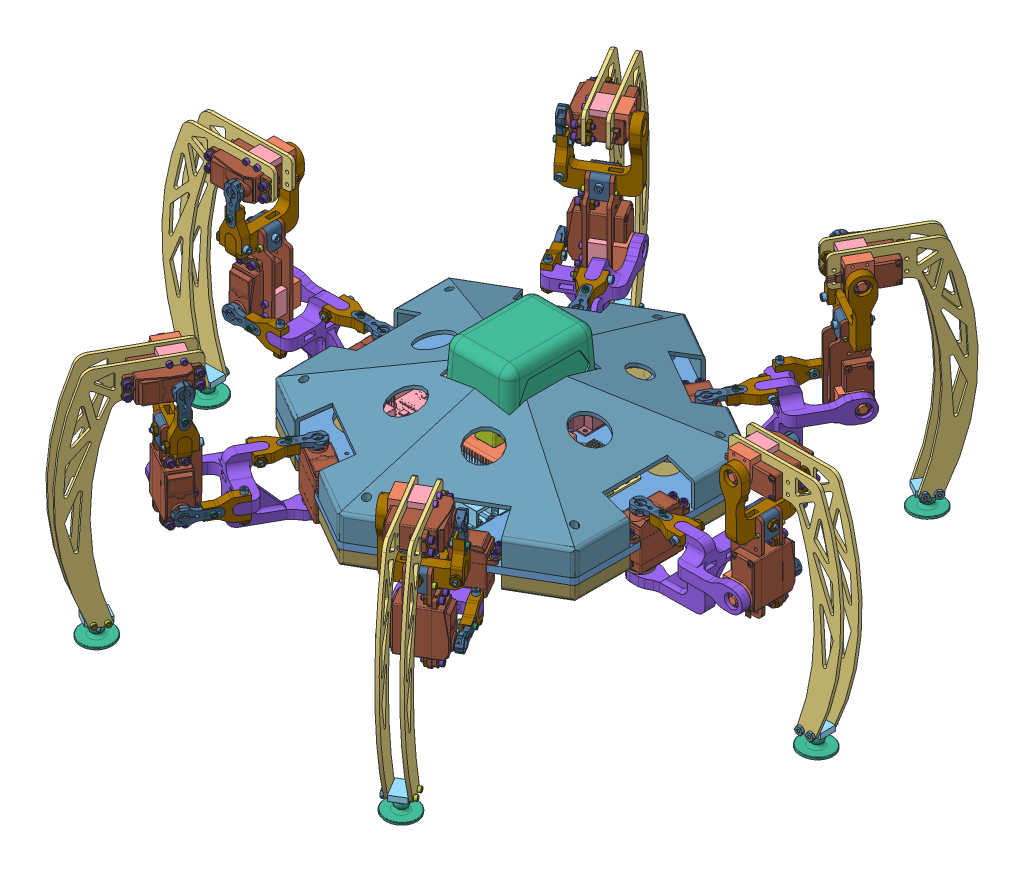
SolidWorks assembly Hexapod_(Hexagonal), configuration Défaut. Lengths in mm. (continued)
Components (placement in the parent): (continued)
- Foot+Tibia+Femur-11: Foot+Tibia+Femur [Défaut] at (-76.9411 -25 -93.0658) x (0.5 0 0.866025) z (-0.866025 0 0.5) size (210.19 223.27 63.83) (flexible)
  - Femur-1: Femur [Défaut] at origin size (137.43 61.64 61.08) (flexible)
    - Joint_(Femur_to_tibia)-1: Joint_(Femur_to_tibia) [Défaut] at (-66.4348 29.5 -48.8085) x (0.999924 0 -0.012321) z (0.012321 0 0.999924) size (122 58.8 58.8)
    - Horn_attachment-3: Horn_attachment [Défaut] at (-38.1979 44.8 -29.755) x (0.999924 0 -0.012321) z (0 1 0) size (33 20 8)
    - Horn-3: Horn [Défaut] at (-10.2 48.8 -30.1) x (-0.999924 0 0.012321) z (0 1 0) size (35.39 15.87 6)
    - DS3225MG-3: DS3225MG [Default] at (-10.2 45.8 -30.1) x (0 0 1) z (0 1 0) size (57.25 20.4 45.91)
    - Bearing_mount_(Femur)-1: Bearing_mount_(Femur) [Default] at (2.5 22 -30.1) x (1 0 0) z (0 -1 0) size (35.3 20.2 31)
    - Bearing-3: Bearing [Default] at (-10.2 -6.7498 -30.1) x (0.400474 0 0.916308) z (-0.916308 0 0.400474) size (13.87 4.75 13.87)
    - MSHXNUT 0.112-40-D-N-1: MSHXNUT 0.112-40-D-N [MSHXNUT 0.112-40-D-N] at (-30.1985 40.8 -29.8536) x (-0.510633 0 -0.859799) z (0 1 0) size (6.35 7.33 2.49)
    - HX-SHCS 0.112-40x0.4375x0.4375-N-1: HX-SHCS 0.112-40x0.4375x0.4375-N [HX-SHCS 0.112-40x0.4375x0.4375-N] at (-30.1985 51.6448 -29.8536) x (0 -1 0) z (-0.489292 0 0.87212) size (13.96 4.65 4.65)
    - Narrow FW 0.138-1: Narrow FW 0.138 [Narrow FW 0.138] at (-15.2 31.2 4.7) x (0 -1 0) z (-0.829316 0 -0.55878) size (0.81 7.92 7.92)
    - HX-SHCS 0.138-32x0.5x0.5-N-1: HX-SHCS 0.138-32x0.5x0.5-N [HX-SHCS 0.138-32x0.5x0.5-N] at (-15.2 35.772 4.7) x (0 -1 0) z (0.866025 0 -0.5) size (16.21 5.74 5.74)
    - Narrow FW 0.138-2: Narrow FW 0.138 [Narrow FW 0.138] at (-15.2 31.2 -44.9) x (0 -1 0) z (-0.829316 0 -0.55878) size (0.81 7.92 7.92)
    - Narrow FW 0.138-3: Narrow FW 0.138 [Narrow FW 0.138] at (-5.2 31.2 4.7) x (0 -1 0) z (-0.829316 0 -0.55878) size (0.81 7.92 7.92)
    - Narrow FW 0.138-4: Narrow FW 0.138 [Narrow FW 0.138] at (-5.2 31.2 -44.9) x (0 -1 0) z (-0.829316 0 -0.55878) size (0.81 7.92 7.92)
    - HX-SHCS 0.138-32x0.5x0.5-N-2: HX-SHCS 0.138-32x0.5x0.5-N [HX-SHCS 0.138-32x0.5x0.5-N] at (-15.2 35.772 -44.9) x (0 -1 0) z (0.866025 0 -0.5) size (16.21 5.74 5.74)
    - HX-SHCS 0.138-32x0.5x0.5-N-3: HX-SHCS 0.138-32x0.5x0.5-N [HX-SHCS 0.138-32x0.5x0.5-N] at (-5.2 35.772 4.7) x (0 -1 0) z (0.866025 0 -0.5) size (16.21 5.74 5.74)
    - HX-SHCS 0.138-32x0.5x0.5-N-4: HX-SHCS 0.138-32x0.5x0.5-N [HX-SHCS 0.138-32x0.5x0.5-N] at (-5.2 35.772 -44.9) x (0 -1 0) z (0.866025 0 -0.5) size (16.21 5.74 5.74)
    - MSHXNUT 0.138-32-D-N-1: MSHXNUT 0.138-32-D-N [MSHXNUT 0.138-32-D-N] at (-52.0379 44.8 -16.6879) x (-0.86596 -0.5 0.010671) z (0.012321 0 0.999924) size (7.92 9.15 2.9)
    - HX-SHCS 0.138-32x1x1-N-2: HX-SHCS 0.138-32x1x1-N [HX-SHCS 0.138-32x1x1-N] at (-52.3632 44.8 -43.0867) x (0.012321 0 0.999924) z (-0.86596 -0.5 0.010671) size (28.91 5.74 5.74)
  - Foot_(Long)-4: Foot_(Long) [Défaut] at (-141.7664 117.7478 -37.8795) x (0.999923 0.001668 -0.012321) z (0.012321 0 0.999924) size (104.1 223.13 60.64) (flexible)
    - DS3225MG-1: DS3225MG [Default] at (30.1 10.2 45.8) x (-1 0 0) z (0 0 1) size (57.25 20.4 45.91)
    - Bearing-1: Bearing [Default] at (30.1 10.2 -6.7498) x (-0.568255 0.822853 0) z (0.822853 0.568255 0) size (13.87 4.75 13.87)
    - Bearing_mount_(Foot)-1: Bearing_mount_(Foot) [Default] at (30.1 22.9 8.1) x (0 1 0) z (0 0 -1) size (25.3 20.2 17.1)
    - Foot_(Long)-1: Foot_(Long) [Default] at (18.7 14 25) size (103.08 208 3)
    - Link-1: Link [Default] at (30.1 22.9 11.1) x (0 -1 0) z (0 0 1) size (5 20.2 13.9)
    - Foot_(Long)-2: Foot_(Long) [Default] at (18.7 14 8.1) size (103.08 208 3)
    - Joint_(Foot_to_slipper)-2: Joint_(Foot_to_slipper) [Default] at (-21.9427 -177.5 11.1) x (0 1 0) z (0 0 1) size (15 20.2 13.9)
    - Horn-1: Horn [Défaut] at (30.1 10.2 48.8) x (-0.007987 -0.999968 0) z (0 0 1) size (35.39 15.87 6)
    - Horn_attachment-1: Horn_attachment [Défaut] at (29.8764 -17.7991 44.8) x (0.007987 0.999968 0) z (0 0 1) size (33 20 8)
    - Slipper-1: Slipper [Défaut] at (-21.7184 -191.9896 17.7406) x (0.999392 0.031392 0.015197) z (-0.013787 -0.044657 0.998907) size (30 10.55 30)
    - HX-SHCS 0.112-40x0.4375x0.4375-N-15: HX-SHCS 0.112-40x0.4375x0.4375-N [HX-SHCS 0.112-40x0.4375x0.4375-N] at (29.9403 -9.7994 51.6448) x (0 0 -1) z (0.869991 0.493067 0) size (13.96 4.65 4.65)
    - MSHXNUT 0.112-40-D-N-7: MSHXNUT 0.112-40-D-N [MSHXNUT 0.112-40-D-N] at (29.9403 -9.7994 40.8) x (-0.007987 -0.999968 0) z (0 0 1) size (6.35 7.33 2.49)
    - HX-SHCS 0.112-40x0.875x0.875-N-9: HX-SHCS 0.112-40x0.875x0.875-N [HX-SHCS 0.112-40x0.875x0.875-N] at (-26.9427 -177.5 30.8448) x (0 0 -1) z (0 1 0) size (25.07 4.65 4.65)
    - MSHXNUT 0.112-40-D-N-4: MSHXNUT 0.112-40-D-N [MSHXNUT 0.112-40-D-N] at (-26.9427 -177.5 8.1) x (0.866025 -0.5 0) z (0 0 1) size (6.35 7.33 2.49)
    - HX-SHCS 0.112-40x0.875x0.875-N-11: HX-SHCS 0.112-40x0.875x0.875-N [HX-SHCS 0.112-40x0.875x0.875-N] at (-16.9427 -177.5 30.8448) x (0 0 -1) z (0 1 0) size (25.07 4.65 4.65)
    - MSHXNUT 0.112-40-D-N-6: MSHXNUT 0.112-40-D-N [MSHXNUT 0.112-40-D-N] at (-16.9427 -177.5 8.1) x (0.866025 -0.5 0) z (0 0 1) size (6.35 7.33 2.49)
    - HX-SHCS 0.112-40x1x0.75-N-13: HX-SHCS 0.112-40x1x0.75-N [HX-SHCS 0.112-40x1x0.75-N] at (25.1 22.9 30.8448) x (0 0 -1) z (0 1 0) size (28.24 4.65 4.65)
    - HX-SHCS 0.112-40x1x0.75-N-14: HX-SHCS 0.112-40x1x0.75-N [HX-SHCS 0.112-40x1x0.75-N] at (35.1 22.9 30.8448) x (0 0 -1) z (0 1 0) size (28.24 4.65 4.65)
    - HX-SHCS 0.138-32x0.5x0.5-N-14: HX-SHCS 0.138-32x0.5x0.5-N [HX-SHCS 0.138-32x0.5x0.5-N] at (-4.7 5.2 35.772) x (0 0 -1) z (0.866025 0.5 0) size (16.21 5.74 5.74)
    - Narrow FW 0.138-1: Narrow FW 0.138 [Narrow FW 0.138] at (-4.7 5.2 31.2) x (0 0 -1) z (-0.829316 0.55878 0) size (0.81 7.92 7.92)
    - MSHXNUT 0.138-32-D-N-1: MSHXNUT 0.138-32-D-N [MSHXNUT 0.138-32-D-N] at (-4.7 5.2 25) x (0.866025 0.5 0) z (0 0 1) size (7.92 9.15 2.9)
    - MSHXNUT 0.138-32-D-N-2: MSHXNUT 0.138-32-D-N [MSHXNUT 0.138-32-D-N] at (44.9 5.2 25) x (0.866025 0.5 0) z (0 0 1) size (7.92 9.15 2.9)
    - MSHXNUT 0.138-32-D-N-3: MSHXNUT 0.138-32-D-N [MSHXNUT 0.138-32-D-N] at (-4.7 15.2 25) x (0.866025 0.5 0) z (0 0 1) size (7.92 9.15 2.9)
    - MSHXNUT 0.138-32-D-N-4: MSHXNUT 0.138-32-D-N [MSHXNUT 0.138-32-D-N] at (44.9 15.2 25) x (0.866025 0.5 0) z (0 0 1) size (7.92 9.15 2.9)
    - HX-SHCS 0.138-32x0.5x0.5-N-15: HX-SHCS 0.138-32x0.5x0.5-N [HX-SHCS 0.138-32x0.5x0.5-N] at (44.9 5.2 35.772) x (0 0 -1) z (0.866025 0.5 0) size (16.21 5.74 5.74)
    - HX-SHCS 0.138-32x0.5x0.5-N-16: HX-SHCS 0.138-32x0.5x0.5-N [HX-SHCS 0.138-32x0.5x0.5-N] at (-4.7 15.2 35.772) x (0 0 -1) z (0.866025 0.5 0) size (16.21 5.74 5.74)
    - HX-SHCS 0.138-32x0.5x0.5-N-17: HX-SHCS 0.138-32x0.5x0.5-N [HX-SHCS 0.138-32x0.5x0.5-N] at (44.9 15.2 35.772) x (0 0 -1) z (0.866025 0.5 0) size (16.21 5.74 5.74)
    - Narrow FW 0.138-2: Narrow FW 0.138 [Narrow FW 0.138] at (44.9 5.2 31.2) x (0 0 -1) z (-0.829316 0.55878 0) size (0.81 7.92 7.92)
    - Narrow FW 0.138-3: Narrow FW 0.138 [Narrow FW 0.138] at (-4.7 15.2 31.2) x (0 0 -1) z (-0.829316 0.55878 0) size (0.81 7.92 7.92)
    - Narrow FW 0.138-4: Narrow FW 0.138 [Narrow FW 0.138] at (44.9 15.2 31.2) x (0 0 -1) z (-0.829316 0.55878 0) size (0.81 7.92 7.92)
  - Tibia-3: Tibia [Défaut] at (-122.5709 19.4647 -38.1161) x (-0.006318 -0.99998 0.000078) z (0.012321 0 0.999924) size (129.02 61.26 61.64) (flexible)
    - Joint_(Tibia_to_foot)-1: Joint_(Tibia_to_foot) [Défaut] at (-62.6 10.2 -10) size (64 20 58.8)
    - DS3225MG-2: DS3225MG [Default] at (-10.1 10.2 45.8) x (-1 0 0) z (0 0 1) size (57.25 20.4 45.91)
    - Link-3: Link [Default] at (-10.1 22.9 11.1) x (0 -1 0) z (0 0 1) size (5 20.2 13.9)
    - Horn-2: Horn [Défaut] at (-10.1 10.2 48.8) x (-0.006319 0.99998 0) z (0 0 1) size (35.39 15.87 6)
    - Horn_attachment-2: Horn_attachment [Défaut] at (-10.2769 38.1994 44.8) x (0.006319 -0.99998 0) z (0 0 1) size (33 20 8)
    - Joint_attachment_(Tibia)-1: Joint_attachment_(Tibia) [Défaut] at (-62.6 10.2 25) size (19 20.4 13.9)
    - Tibia-1: Tibia [Défaut] at (-62.6 10.2 28) size (80 28 3)
    - Tibia-2: Tibia [Défaut] at (-62.6 10.2 11.1) size (80 28 3)
    - Bearing_mount_(Foot)-2: Bearing_mount_(Foot) [Default] at (-10.1 22.9 8.1) x (0 1 0) z (0 0 -1) size (25.3 20.2 17.1)
    - Bearing-2: Bearing [Default] at (-10.1 10.2 -6.7498) x (-0.993915 0.110147 0) z (0.110147 0.993915 0) size (13.87 4.75 13.87)
    - HX-SHCS 0.112-40x0.4375x0.4375-N-1: HX-SHCS 0.112-40x0.4375x0.4375-N [HX-SHCS 0.112-40x0.4375x0.4375-N] at (-10.2264 30.1996 51.6448) x (0 0 -1) z (-0.862849 -0.505462 0) size (13.96 4.65 4.65)
    - MSHXNUT 0.112-40-D-N-1: MSHXNUT 0.112-40-D-N [MSHXNUT 0.112-40-D-N] at (-10.2264 30.1996 40.8) x (-0.006319 0.99998 0) z (0 0 1) size (6.35 7.33 2.49)
    - HX-SHCS 0.112-40x1x0.75-N-1: HX-SHCS 0.112-40x1x0.75-N [HX-SHCS 0.112-40x1x0.75-N] at (-15.1 22.9 30.8448) x (0 0 -1) z (0 1 0) size (28.24 4.65 4.65)
    - HX-SHCS 0.112-40x1x0.75-N-2: HX-SHCS 0.112-40x1x0.75-N [HX-SHCS 0.112-40x1x0.75-N] at (-5.1 22.9 30.8448) x (0 0 -1) z (0 1 0) size (28.24 4.65 4.65)
    - HX-SHCS 0.138-32x0.5x0.5-N-1: HX-SHCS 0.138-32x0.5x0.5-N [HX-SHCS 0.138-32x0.5x0.5-N] at (-44.9 5.2 35.772) x (0 0 -1) z (0.866025 0.5 0) size (16.21 5.74 5.74)
    - Narrow FW 0.138-1: Narrow FW 0.138 [Narrow FW 0.138] at (-44.9 5.2 31.2) x (0 0 -1) z (-0.54947 -0.835514 0) size (0.81 7.92 7.92)
    - MSHXNUT 0.138-32-D-N-1: MSHXNUT 0.138-32-D-N [MSHXNUT 0.138-32-D-N] at (-44.9 5.2 25) x (0.866025 0.5 0) z (0 0 1) size (7.92 9.15 2.9)
    - MSHXNUT 0.138-32-D-N-2: MSHXNUT 0.138-32-D-N [MSHXNUT 0.138-32-D-N] at (4.7 5.2 25) x (0.866025 0.5 0) z (0 0 1) size (7.92 9.15 2.9)
    - MSHXNUT 0.138-32-D-N-3: MSHXNUT 0.138-32-D-N [MSHXNUT 0.138-32-D-N] at (-44.9 15.2 25) x (0.866025 0.5 0) z (0 0 1) size (7.92 9.15 2.9)
    - MSHXNUT 0.138-32-D-N-4: MSHXNUT 0.138-32-D-N [MSHXNUT 0.138-32-D-N] at (4.7 15.2 25) x (0.866025 0.5 0) z (0 0 1) size (7.92 9.15 2.9)
    - Narrow FW 0.138-2: Narrow FW 0.138 [Narrow FW 0.138] at (4.7 5.2 31.2) x (0 0 -1) z (-0.54947 -0.835514 0) size (0.81 7.92 7.92)
    - Narrow FW 0.138-3: Narrow FW 0.138 [Narrow FW 0.138] at (-44.9 15.2 31.2) x (0 0 -1) z (-0.54947 -0.835514 0) size (0.81 7.92 7.92)
    - Narrow FW 0.138-4: Narrow FW 0.138 [Narrow FW 0.138] at (4.7 15.2 31.2) x (0 0 -1) z (-0.54947 -0.835514 0) size (0.81 7.92 7.92)
    - HX-SHCS 0.138-32x0.5x0.5-N-2: HX-SHCS 0.138-32x0.5x0.5-N [HX-SHCS 0.138-32x0.5x0.5-N] at (4.7 5.2 35.772) x (0 0 -1) z (0.866025 0.5 0) size (16.21 5.74 5.74)
    - HX-SHCS 0.138-32x0.5x0.5-N-3: HX-SHCS 0.138-32x0.5x0.5-N [HX-SHCS 0.138-32x0.5x0.5-N] at (-44.9 15.2 35.772) x (0 0 -1) z (0.866025 0.5 0) size (16.21 5.74 5.74)
    - HX-SHCS 0.138-32x0.5x0.5-N-4: HX-SHCS 0.138-32x0.5x0.5-N [HX-SHCS 0.138-32x0.5x0.5-N] at (4.7 15.2 35.772) x (0 0 -1) z (0.866025 0.5 0) size (16.21 5.74 5.74)
    - HX-SHCS 0.112-40x0.875x0.875-N-1: HX-SHCS 0.112-40x0.875x0.875-N [HX-SHCS 0.112-40x0.875x0.875-N] at (-57.6 17.8 30.8448) x (0 0 -1) z (0 1 0) size (25.07 4.65 4.65)
    - HX-SHCS 0.112-40x0.875x0.875-N-2: HX-SHCS 0.112-40x0.875x0.875-N [HX-SHCS 0.112-40x0.875x0.875-N] at (-57.6 2.6 30.8448) x (0 0 -1) z (0 1 0) size (25.07 4.65 4.65)
    - HX-SHCS 0.138-32x1x1-N-1: HX-SHCS 0.138-32x1x1-N [HX-SHCS 0.138-32x1x1-N] at (-62.6 23.9052 18.05) x (0 -1 0) z (1 0 0) size (28.91 5.74 5.74)
    - MSHXNUT 0.138-32-D-N-5: MSHXNUT 0.138-32-D-N [MSHXNUT 0.138-32-D-N] at (-62.6 -2.8956 18.05) x (1 0 0) z (0 -1 0) size (7.92 9.15 2.9)
  - HX-SHCS 0.138-32x1x1-N-1: HX-SHCS 0.138-32x1x1-N [HX-SHCS 0.138-32x1x1-N] at (-69.7593 43.0052 6.0366) x (0 -1 0) z (-0.87212 0 -0.489292) size (28.91 5.74 5.74)
  - MSHXNUT 0.138-32-D-N-1: MSHXNUT 0.138-32-D-N [MSHXNUT 0.138-32-D-N] at (-69.7593 16.6044 6.0366) x (-0.87212 0 -0.489292) z (0 -1 0) size (7.92 9.15 2.9)
  - MSHXNUT 0.138-32-D-N-2: MSHXNUT 0.138-32-D-N [MSHXNUT 0.138-32-D-N] at (-124.2935 86.0804 6.7086) x (-0.000689 0.866008 -0.500029) z (-0.999904 0.006319 0.012321) size (7.92 9.15 2.9)
  - HX-SHCS 0.138-32x1x1-N-2: HX-SHCS 0.138-32x1x1-N [HX-SHCS 0.138-32x1x1-N] at (-97.8952 85.9135 6.3833) x (-0.999904 0.006319 0.012321) z (-0.012321 0 -0.999924) size (28.91 5.74 5.74)
- Shell_(Bottom)-1: Shell_(Bottom) [Défaut] at (0 -3 0) x (1 0 0) z (0 0 -1) size (278.74 30 320)
- DROK_090483-1: DROK_090483 [Défaut] at (30 3 -38.21) x (0 0 -1) z (0 1 0) size (50.02 60 18.9)
- Shell_(Top)-1: Shell_(Top) [Défaut] at (0 3 0) size (278.74 60.1 320)
- HX-SHCS 0.138-32x0.5x0.5-N-1: HX-SHCS 0.138-32x0.5x0.5-N [HX-SHCS 0.138-32x0.5x0.5-N] at (-123.7436 6.5052 -65.6699) x (0 -1 0) z (0 0 1) size (16.21 5.74 5.74)
- HX-SHCS 0.138-32x0.5x0.5-N-2: HX-SHCS 0.138-32x0.5x0.5-N [HX-SHCS 0.138-32x0.5x0.5-N] at (-118.7436 6.5052 74.3301) x (0 -1 0) z (0.866025 0 0.5) size (16.21 5.74 5.74)
- HX-SHCS 0.138-32x0.5x0.5-N-3: HX-SHCS 0.138-32x0.5x0.5-N [HX-SHCS 0.138-32x0.5x0.5-N] at (5 6.5052 140) x (0 -1 0) z (0.866025 0 -0.5) size (16.21 5.74 5.74)
- HX-SHCS 0.138-32x0.5x0.5-N-4: HX-SHCS 0.138-32x0.5x0.5-N [HX-SHCS 0.138-32x0.5x0.5-N] at (123.7436 6.5052 65.6699) x (0 -1 0) z (0 0 -1) size (16.21 5.74 5.74)
- HX-SHCS 0.138-32x0.5x0.5-N-5: HX-SHCS 0.138-32x0.5x0.5-N [HX-SHCS 0.138-32x0.5x0.5-N] at (118.7436 6.5052 -74.3301) x (0 -1 0) z (-0.866025 0 -0.5) size (16.21 5.74 5.74)
- HX-SHCS 0.138-32x0.5x0.5-N-6: HX-SHCS 0.138-32x0.5x0.5-N [HX-SHCS 0.138-32x0.5x0.5-N] at (-5 6.5052 -140) x (0 -1 0) z (-0.866025 0 0.5) size (16.21 5.74 5.74)
- HX-SHCS 0.138-32x0.5x0.5-N-7: HX-SHCS 0.138-32x0.5x0.5-N [HX-SHCS 0.138-32x0.5x0.5-N] at (-123.7436 -6.5052 65.6699) x (0 1 0) z (0.866025 0 -0.5) size (16.21 5.74 5.74)
- HX-SHCS 0.138-32x0.5x0.5-N-8: HX-SHCS 0.138-32x0.5x0.5-N [HX-SHCS 0.138-32x0.5x0.5-N] at (-5 -6.5052 140) x (0 1 0) z (0 0 -1) size (16.21 5.74 5.74)
- HX-SHCS 0.138-32x0.5x0.5-N-9: HX-SHCS 0.138-32x0.5x0.5-N [HX-SHCS 0.138-32x0.5x0.5-N] at (118.7436 -6.5052 74.3301) x (0 1 0) z (-0.866025 0 -0.5) size (16.21 5.74 5.74)
- HX-SHCS 0.138-32x0.5x0.5-N-10: HX-SHCS 0.138-32x0.5x0.5-N [HX-SHCS 0.138-32x0.5x0.5-N] at (123.7436 -6.5052 -65.6699) x (0 1 0) z (-0.866025 0 0.5) size (16.21 5.74 5.74)
- HX-SHCS 0.138-32x0.5x0.5-N-11: HX-SHCS 0.138-32x0.5x0.5-N [HX-SHCS 0.138-32x0.5x0.5-N] at (5 -6.5052 -140) x (0 1 0) z (0 0 1) size (16.21 5.74 5.74)
- HX-SHCS 0.138-32x0.5x0.5-N-12: HX-SHCS 0.138-32x0.5x0.5-N [HX-SHCS 0.138-32x0.5x0.5-N] at (-118.7436 -6.5052 -74.3301) x (0 1 0) z (0.866025 0 0.5) size (16.21 5.74 5.74)
Mates (geometry in assembly coordinates):
- Concentric9: concentric aligned: cylinder of Body_(Hexagonal)-1 through (-24.675 -3 24.675) axis (0 1 0) radius 1.45; cylinder of Battery_holder-1 through (-24.675 3 24.675) axis (0 1 0) radius 1.45
- Concentric10: concentric aligned: cylinder of Body_(Hexagonal)-1 through (24.675 -3 -24.675) axis (0 1 0) radius 1.45; cylinder of Battery_holder-1 through (24.675 3 -24.675) axis (0 1 0) radius 1.45
- Coincident1: coincident anti-aligned: plane of Body_(Hexagonal)-1 through (-133.3679 3 -77) normal (0 1 0); plane of 12Channel PWM-2 through (56.8 3 -27.95) normal (0 -1 0)
- Concentric11: concentric aligned: cylinder of Body_(Hexagonal)-1 through (56.8 -3 -27.95) axis (0 1 0) radius 1.25; cylinder of 12Channel PWM-2 through (56.8 -0.5355 -27.95) axis (0 1 0) radius 1.25
- Concentric12: concentric aligned: cylinder of Body_(Hexagonal)-1 through (38 -3 27.95) axis (0 1 0) radius 1.25; cylinder of 12Channel PWM-2 through (38 -0.5355 27.95) axis (0 1 0) radius 1.25
- Coincident2: coincident anti-aligned: plane of Body_(Hexagonal)-1 through (-133.3679 3 -77) normal (0 1 0); plane of 12Channel PWM-1 through (86.9 3 -27.95) normal (0 -1 0)
- Concentric13: concentric aligned: cylinder of Body_(Hexagonal)-1 through (86.9 -3 -27.95) axis (0 1 0) radius 1.25; cylinder of 12Channel PWM-1 through (86.9 -0.5355 -27.95) axis (0 1 0) radius 1.25
- Concentric14: concentric aligned: cylinder of Body_(Hexagonal)-1 through (68.1 -3 27.95) axis (0 1 0) radius 1.25; cylinder of 12Channel PWM-1 through (68.1 -0.5355 27.95) axis (0 1 0) radius 1.25
- Coincident5: coincident anti-aligned: plane of Body_(Hexagonal)-1 through (-133.3679 3 -77) normal (0 1 0); plane of arduinoMega-2 through (-61.35 3 1.27) normal (0 -1 0)
- Concentric15: concentric aligned: cylinder of Body_(Hexagonal)-1 through (-85.46 -3 35.53) axis (0 1 0) radius 1.45; cylinder of arduinoMega-2 through (-85.46 5 35.53) axis (0 1 0) radius 1.6
- Concentric16: concentric aligned: cylinder of Body_(Hexagonal)-1 through (-37.24 -3 -45.71) axis (0 1 0) radius 1.45; cylinder of arduinoMega-2 through (-37.24 5 -45.71) axis (0 1 0) radius 1.6
- Concentric17: concentric aligned: cylinder of Body_(Hexagonal)-1 through (-26.5 -3 39.45) axis (0 1 0) radius 1.375; cylinder of raspberryPi3B-1 through (-26.5 5.5 39.45) axis (0 1 0) radius 1.375
- Concentric18: concentric aligned: cylinder of Body_(Hexagonal)-1 through (31.5 -3 88.45) axis (0 1 0) radius 1.375; cylinder of raspberryPi3B-1 through (31.5 5.5 88.45) axis (0 1 0) radius 1.375
- Coincident11: coincident anti-aligned: plane of Body_(Hexagonal)-1 through (-133.3679 3 -77) normal (0 1 0); plane of raspberryPi3B-1 through (12.5 3 63.95) normal (0 -1 0)
- Coincident13: coincident anti-aligned: plane of Battery_holder-1 through (-15 22.6 15) normal (0 1 0); plane of Battery-1/MAKITA 4.0AH MOBILE-1 through (17.4625 22.6 25.1631) normal (0 -1 0)
- Parallel4: parallel anti-aligned: line of Battery_holder-1 through (-11 20.975 14.8295) axis (1 0 0); line of Battery-1/MAKITA 4.0AH MOBILE-1 through (8.7312 22.6 15) axis (-1 0 0)
- Distance7: distance = 1.475 mm anti-aligned: plane of Battery-1/MAKITA 4.0AH MOBILE-1 through (9.525 20.9552 11.759) normal (1 0 0); plane of Battery_holder-1 through (11 9.35 15) normal (-1 0 0)
- Coincident17: coincident: plane of Battery_holder-1 through (0 14.35 15) normal (0 0 1); line of Battery-1/MAKITA 4.0AH MOBILE-1 through (8.7312 22.6 15) axis (-1 0 0)
- Coincident18: coincident anti-aligned: plane of Body_(Hexagonal)-1 through (-133.3679 3 -77) normal (0 1 0); plane of Battery_holder-1 through (-15 3 15) normal (0 -1 0)
- Concentric21: concentric anti-aligned: cylinder of Body_(Hexagonal)-1 through (-134.2679 -3 -24.8) axis (0 1 0) radius 1.45; cylinder of Foot+Tibia+Femur-1/DS3225MG-3 through (-134.2679 20.8 -24.8) axis (0 -1 0) radius 2.25
- Concentric22: concentric anti-aligned: cylinder of Body_(Hexagonal)-1 through (-124.2679 -3 24.8) axis (0 1 0) radius 1.45; cylinder of Foot+Tibia+Femur-1/DS3225MG-3 through (-124.2679 20.8 24.8) axis (0 -1 0) radius 2.25
- Coincident19: coincident anti-aligned: plane of Body_(Hexagonal)-1 through (-133.3679 3 -77) normal (0 1 0); plane of Foot+Tibia+Femur-1/DS3225MG-3 through (-138.4679 3 -19.1) normal (0 -1 0)
- Concentric23: concentric anti-aligned: cylinder of Body_(Hexagonal)-1 through (-83.6114 -3 -95.2192) axis (0 1 0) radius 1.45; cylinder of Foot+Tibia+Femur-2/DS3225MG-3 through (-83.6114 20.8 -95.2192) axis (0 -1 0) radius 2.25
- Concentric24: concentric anti-aligned: cylinder of Body_(Hexagonal)-1 through (-45.6565 -3 -128.6794) axis (0 1 0) radius 1.45; cylinder of Foot+Tibia+Femur-2/DS3225MG-3 through (-45.6565 20.8 -128.6794) axis (0 -1 0) radius 2.25
- Coincident20: coincident anti-aligned: plane of Body_(Hexagonal)-1 through (-133.3679 3 -77) normal (0 1 0); plane of Foot+Tibia+Femur-2/DS3225MG-3 through (-52.6929 3 -129.4667) normal (0 -1 0)
- Coincident25: coincident anti-aligned: plane of Body_(Hexagonal)-1 through (-133.3679 -3 -77) normal (0 -1 0); plane of Shell_(Bottom)-1 through (-133.3679 -3 -77) normal (0 1 0)
- Concentric25: concentric anti-aligned: cylinder of Body_(Hexagonal)-1 through (-123.7436 3 -65.6699) axis (0 -1 0) radius 1.45; cylinder of Shell_(Bottom)-1 through (-123.7436 -30.4538 -65.6699) axis (0 1 0) radius 1.45
- Concentric26: concentric anti-aligned: cylinder of Body_(Hexagonal)-1 through (-123.7436 3 65.6699) axis (0 -1 0) radius 1.45; cylinder of Shell_(Bottom)-1 through (-123.7436 -30.4538 65.6699) axis (0 1 0) radius 3.4
- Concentric29: concentric aligned: cylinder of Body_(Hexagonal)-1 through (26.415 -3 -41.395) axis (0 1 0) radius 1.45; cylinder of DROK_090483-1 through (26.415 3 -41.395) axis (0 1 0) radius 1.585
- Concentric30: concentric aligned: cylinder of Body_(Hexagonal)-1 through (-26.415 -3 -78.025) axis (0 1 0) radius 1.45; cylinder of DROK_090483-1 through (-26.415 3 -78.025) axis (0 1 0) radius 1.585
- Coincident27: coincident anti-aligned: plane of Body_(Hexagonal)-1 through (-133.3679 3 -77) normal (0 1 0); plane of DROK_090483-1 through (0 3 -59.71) normal (0 -1 0)
- Coincident28: coincident anti-aligned: plane of Body_(Hexagonal)-1 through (-133.3679 3 -77) normal (0 1 0); plane of Shell_(Top)-1 through (-133.3679 3 77) normal (0 -1 0)
- Concentric31: concentric aligned: cylinder of Body_(Hexagonal)-1 through (-123.7436 3 65.6699) axis (0 -1 0) radius 1.45; cylinder of Shell_(Top)-1 through (-123.7436 43.765 65.6699) axis (0 -1 0) radius 1.45
- Concentric32: concentric aligned: cylinder of Body_(Hexagonal)-1 through (-123.7436 3 -65.6699) axis (0 -1 0) radius 1.45; cylinder of Shell_(Top)-1 through (-123.7436 43.765 -65.6699) axis (0 -1 0) radius 3.4
- Coincident29: coincident anti-aligned: plane of Body_(Hexagonal)-1 through (-133.3679 3 -77) normal (0 1 0); plane of HX-SHCS 0.138-32x0.5x0.5-N-1 through (-120.8734 3 -65.6699) normal (0 -1 0)
- Concentric33: concentric anti-aligned: cylinder of Shell_(Top)-1 through (-123.7436 43.765 -65.6699) axis (0 -1 0) radius 3.4; cylinder of HX-SHCS 0.138-32x0.5x0.5-N-1 through (-123.7436 38.2552 -65.6699) axis (0 1 0) radius 1.7526
- Coincident30: coincident anti-aligned: plane of Body_(Hexagonal)-1 through (-133.3679 -3 -77) normal (0 -1 0); plane of HX-SHCS 0.138-32x0.5x0.5-N-7 through (-122.3085 -3 68.1555) normal (0 1 0)
- Concentric34: concentric anti-aligned: cylinder of Shell_(Bottom)-1 through (-123.7436 -30.4538 65.6699) axis (0 1 0) radius 3.4; cylinder of HX-SHCS 0.138-32x0.5x0.5-N-7 through (-123.7436 -38.2552 65.6699) axis (0 -1 0) radius 1.7526
